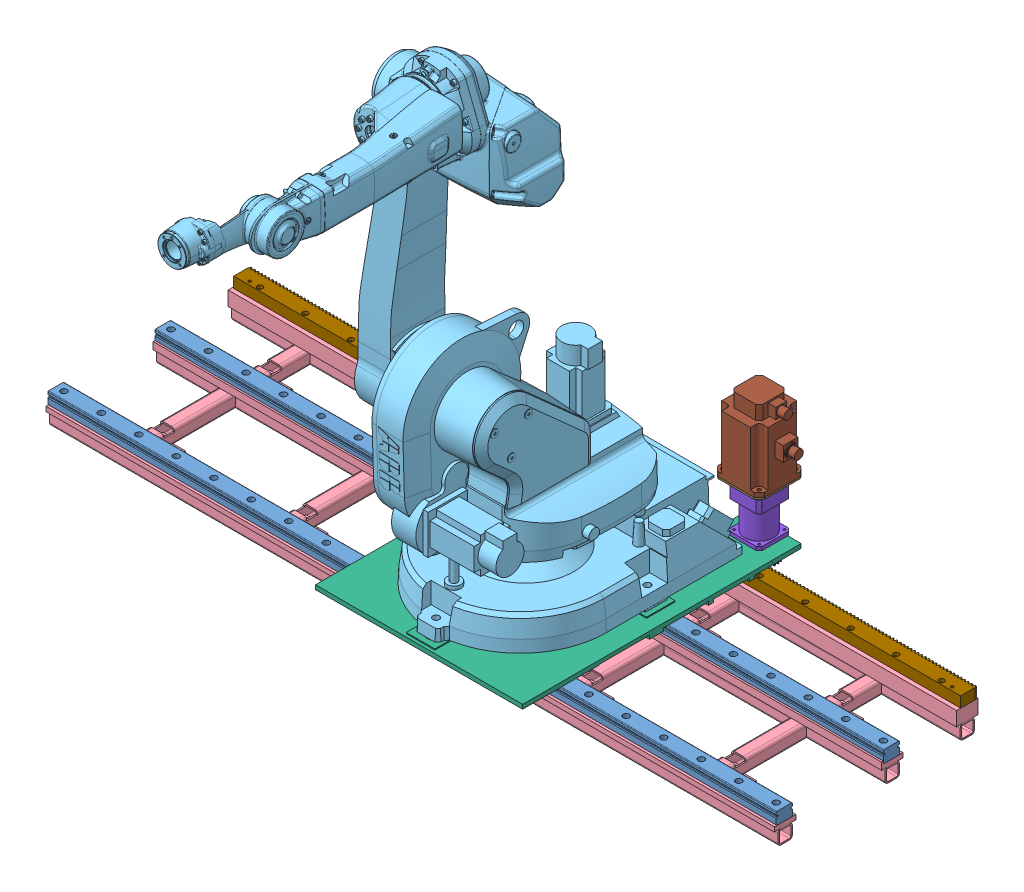
SolidWorks assembly 双导轨, configuration 默认. Lengths in mm.
Overall size (2040.11 1530 1501.91).
62 component instances, 12 part files, 57 mates.
Components (placement in the parent):
- 滑轨-1: 滑轨 [默认] at (-1407.5567 207.206 0) size (2040 34 45)
- 滑轨-2: 滑轨 [默认] at (632.4433 207.206 -300) x (-1 0 0) z (0 0 -1) size (2040 34 45)
- 带螺钉M4滑块-1: 带螺钉M4滑块 [默认] at (-58.6161 241.6075 -300) size (138.91 46.33 120)
  - 滑块-1: 滑块 [默认] at (-71.6389 25.5985 0) size (136 46 120)
  - cross recessed round head wood screws gb-2: cross recessed round head wood screws gb [GB_WOOD_SCREWS_TYPE136 M4X18-N] at (-74.5889 20.6207 -35.126) size (20.91 7.65 7.65)
  - cross recessed round head wood screws gb-4: cross recessed round head wood screws gb [GB_WOOD_SCREWS_TYPE136 M4X18-N] at (-74.5889 -15.566 -35.2553) size (20.91 7.65 7.65)
  - cross recessed round head wood screws gb-5: cross recessed round head wood screws gb [GB_WOOD_SCREWS_TYPE136 M4X18-N] at (-74.5889 20.0027 35.5979) size (20.91 7.65 7.65)
  - cross recessed round head wood screws gb-7: cross recessed round head wood screws gb [GB_WOOD_SCREWS_TYPE136 M4X18-N] at (-74.5889 -15.4341 35.4668) size (20.91 7.65 7.65)
  - cross recessed round head wood screws gb-8: cross recessed round head wood screws gb [GB_WOOD_SCREWS_TYPE136 M4X18-N] at (56.3111 20.1247 35.1143) x (-1 0 0) z (0 -0.924225 -0.381849) size (20.91 7.65 7.65)
  - cross recessed round head wood screws gb-9: cross recessed round head wood screws gb [GB_WOOD_SCREWS_TYPE136 M4X18-N] at (56.3111 -15.3216 35.4319) x (-1 0 0) z (0 -0.924225 -0.381849) size (20.91 7.65 7.65)
  - cross recessed round head wood screws gb-10: cross recessed round head wood screws gb [GB_WOOD_SCREWS_TYPE136 M4X18-N] at (56.3111 19.9496 -35.3218) x (-1 0 0) z (0 -0.924225 -0.381849) size (20.91 7.65 7.65)
  - cross recessed round head wood screws gb-11: cross recessed round head wood screws gb [GB_WOOD_SCREWS_TYPE136 M4X18-N] at (56.3111 -15.7298 -35.1914) x (-1 0 0) z (0 -0.924225 -0.381849) size (20.91 7.65 7.65)
- 带螺钉M4滑块-3: 带螺钉M4滑块 [默认] at (-58.6161 241.6075 0) size (138.91 46.33 120)
  - 滑块-1: 滑块 [默认] at (-71.6389 25.5985 0) size (136 46 120)
  - cross recessed round head wood screws gb-2: cross recessed round head wood screws gb [GB_WOOD_SCREWS_TYPE136 M4X18-N] at (-74.5889 20.6207 -35.126) size (20.91 7.65 7.65)
  - cross recessed round head wood screws gb-4: cross recessed round head wood screws gb [GB_WOOD_SCREWS_TYPE136 M4X18-N] at (-74.5889 -15.566 -35.2553) size (20.91 7.65 7.65)
  - cross recessed round head wood screws gb-5: cross recessed round head wood screws gb [GB_WOOD_SCREWS_TYPE136 M4X18-N] at (-74.5889 20.0027 35.5979) size (20.91 7.65 7.65)
  - cross recessed round head wood screws gb-7: cross recessed round head wood screws gb [GB_WOOD_SCREWS_TYPE136 M4X18-N] at (-74.5889 -15.4341 35.4668) size (20.91 7.65 7.65)
  - cross recessed round head wood screws gb-8: cross recessed round head wood screws gb [GB_WOOD_SCREWS_TYPE136 M4X18-N] at (56.3111 20.1247 35.1143) x (-1 0 0) z (0 -0.924225 -0.381849) size (20.91 7.65 7.65)
  - cross recessed round head wood screws gb-9: cross recessed round head wood screws gb [GB_WOOD_SCREWS_TYPE136 M4X18-N] at (56.3111 -15.3216 35.4319) x (-1 0 0) z (0 -0.924225 -0.381849) size (20.91 7.65 7.65)
  - cross recessed round head wood screws gb-10: cross recessed round head wood screws gb [GB_WOOD_SCREWS_TYPE136 M4X18-N] at (56.3111 19.9496 -35.3218) x (-1 0 0) z (0 -0.924225 -0.381849) size (20.91 7.65 7.65)
  - cross recessed round head wood screws gb-11: cross recessed round head wood screws gb [GB_WOOD_SCREWS_TYPE136 M4X18-N] at (56.3111 -15.7298 -35.1914) x (-1 0 0) z (0 -0.924225 -0.381849) size (20.91 7.65 7.65)
- 带螺钉M4滑块-4: 带螺钉M4滑块 [默认] at (-401.8938 241.6075 0) x (-1 0 0) z (0 0 -1) size (138.91 46.33 120)
  - 滑块-1: 滑块 [默认] at (-71.6389 25.5985 0) size (136 46 120)
  - cross recessed round head wood screws gb-2: cross recessed round head wood screws gb [GB_WOOD_SCREWS_TYPE136 M4X18-N] at (-74.5889 20.6207 -35.126) size (20.91 7.65 7.65)
  - cross recessed round head wood screws gb-4: cross recessed round head wood screws gb [GB_WOOD_SCREWS_TYPE136 M4X18-N] at (-74.5889 -15.566 -35.2553) size (20.91 7.65 7.65)
  - cross recessed round head wood screws gb-5: cross recessed round head wood screws gb [GB_WOOD_SCREWS_TYPE136 M4X18-N] at (-74.5889 20.0027 35.5979) size (20.91 7.65 7.65)
  - cross recessed round head wood screws gb-7: cross recessed round head wood screws gb [GB_WOOD_SCREWS_TYPE136 M4X18-N] at (-74.5889 -15.4341 35.4668) size (20.91 7.65 7.65)
  - cross recessed round head wood screws gb-8: cross recessed round head wood screws gb [GB_WOOD_SCREWS_TYPE136 M4X18-N] at (56.3111 20.1247 35.1143) x (-1 0 0) z (0 -0.924225 -0.381849) size (20.91 7.65 7.65)
  - cross recessed round head wood screws gb-9: cross recessed round head wood screws gb [GB_WOOD_SCREWS_TYPE136 M4X18-N] at (56.3111 -15.3216 35.4319) x (-1 0 0) z (0 -0.924225 -0.381849) size (20.91 7.65 7.65)
  - cross recessed round head wood screws gb-10: cross recessed round head wood screws gb [GB_WOOD_SCREWS_TYPE136 M4X18-N] at (56.3111 19.9496 -35.3218) x (-1 0 0) z (0 -0.924225 -0.381849) size (20.91 7.65 7.65)
  - cross recessed round head wood screws gb-11: cross recessed round head wood screws gb [GB_WOOD_SCREWS_TYPE136 M4X18-N] at (56.3111 -15.7298 -35.1914) x (-1 0 0) z (0 -0.924225 -0.381849) size (20.91 7.65 7.65)
- 带螺钉M4滑块-5: 带螺钉M4滑块 [默认] at (-401.8938 241.6075 -300) x (-1 0 0) z (0 0 -1) size (138.91 46.33 120)
  - 滑块-1: 滑块 [默认] at (-71.6389 25.5985 0) size (136 46 120)
  - cross recessed round head wood screws gb-2: cross recessed round head wood screws gb [GB_WOOD_SCREWS_TYPE136 M4X18-N] at (-74.5889 20.6207 -35.126) size (20.91 7.65 7.65)
  - cross recessed round head wood screws gb-4: cross recessed round head wood screws gb [GB_WOOD_SCREWS_TYPE136 M4X18-N] at (-74.5889 -15.566 -35.2553) size (20.91 7.65 7.65)
  - cross recessed round head wood screws gb-5: cross recessed round head wood screws gb [GB_WOOD_SCREWS_TYPE136 M4X18-N] at (-74.5889 20.0027 35.5979) size (20.91 7.65 7.65)
  - cross recessed round head wood screws gb-7: cross recessed round head wood screws gb [GB_WOOD_SCREWS_TYPE136 M4X18-N] at (-74.5889 -15.4341 35.4668) size (20.91 7.65 7.65)
  - cross recessed round head wood screws gb-8: cross recessed round head wood screws gb [GB_WOOD_SCREWS_TYPE136 M4X18-N] at (56.3111 20.1247 35.1143) x (-1 0 0) z (0 -0.924225 -0.381849) size (20.91 7.65 7.65)
  - cross recessed round head wood screws gb-9: cross recessed round head wood screws gb [GB_WOOD_SCREWS_TYPE136 M4X18-N] at (56.3111 -15.3216 35.4319) x (-1 0 0) z (0 -0.924225 -0.381849) size (20.91 7.65 7.65)
  - cross recessed round head wood screws gb-10: cross recessed round head wood screws gb [GB_WOOD_SCREWS_TYPE136 M4X18-N] at (56.3111 19.9496 -35.3218) x (-1 0 0) z (0 -0.924225 -0.381849) size (20.91 7.65 7.65)
  - cross recessed round head wood screws gb-11: cross recessed round head wood screws gb [GB_WOOD_SCREWS_TYPE136 M4X18-N] at (56.3111 -15.7298 -35.1914) x (-1 0 0) z (0 -0.924225 -0.381849) size (20.91 7.65 7.65)
- 焊架-1: 焊架 [默认<按加工>] at (-1407.5567 174.206 -302.5) x (1 0 0) z (0 1 0) size (2040 570 90)
- 机器人+工件台-1: 机器人+工件台 [默认] at (-235.255 279.206 -245) x (0 0 -1) z (0 1 0) size (1471.91 580 1415)
  - IRB1600ID_4_150__02_STEP_c-1: IRB1600ID_4_150__02_STEP_c [默认] at (-101.9143 0.2591 3) x (-1 0 0) z (0 0 1) size (1372.28 510.23 1392)
  - 工件台-2: 工件台 [默认] at (-50 0 -20) x (1 0 0) z (0 -1 0) size (780 23 580)
- slotted set screws with cone point gb-18: slotted set screws with cone point gb [GB_FASTENER_SCREWS_NCOB M4X16-S] at (-90.255 263.206 -376) x (0 0 1) z (0.748487 -0.66315 0) size (15.99 4 4)
- slotted set screws with cone point gb-16: slotted set screws with cone point gb [GB_FASTENER_SCREWS_NCOB M4X16-S] at (-30.255 263.206 -376) x (0 0 1) z (0.08595 -0.996299 0) size (15.99 4 4)
- slotted set screws with cone point gb-15: slotted set screws with cone point gb [GB_FASTENER_SCREWS_NCOB M4X16-S] at (-50.255 263.206 -376) x (0 0 1) z (-0.998235 -0.059386 0) size (15.99 4 4)
- slotted set screws with cone point gb-13: slotted set screws with cone point gb [GB_FASTENER_SCREWS_NCOB M4X16-S] at (-70.255 263.206 -376) x (0 0 1) z (-0.354194 -0.935172 0) size (15.99 4 4)
- slotted set screws with cone point gb-11: slotted set screws with cone point gb [GB_FASTENER_SCREWS_NCOB M4X16-S] at (-110.255 263.206 -376) x (0 0 1) z (-0.974836 -0.222922 0) size (15.99 4 4)
- slotted set screws with cone point gb-10: slotted set screws with cone point gb [GB_FASTENER_SCREWS_NCOB M4X16-S] at (-435.255 263.206 -376) x (0 0 1) z (-0.993007 0.118057 0) size (15.99 4 4)
- slotted set screws with cone point gb-9: slotted set screws with cone point gb [GB_FASTENER_SCREWS_NCOB M4X16-S] at (-415.255 263.206 -376) x (0 0 1) z (-0.998721 -0.050563 0) size (15.99 4 4)
- slotted set screws with cone point gb-7: slotted set screws with cone point gb [GB_FASTENER_SCREWS_NCOB M4X16-S] at (-395.255 263.206 -376) x (0 0 1) z (-1 0 0) size (15.99 4 4)
- slotted set screws with cone point gb-4: slotted set screws with cone point gb [GB_FASTENER_SCREWS_NCOB M4X16-S] at (-375.255 263.206 -376) x (0 0 1) z (-0.982111 0.188301 0) size (15.99 4 4)
- slotted set screws with cone point gb-2: slotted set screws with cone point gb [GB_FASTENER_SCREWS_NCOB M4X16-S] at (-355.255 263.206 -376) x (0 0 1) z (-0.85186 0.52377 0) size (15.99 4 4)
- PLE8090级数2减速比15-1: PLE8090级数2减速比15 [默认] at (-22.7544 284.206 -585) x (0 -1 0) z (1 0 0) size (162.5 90 90)
- 齿条-2: 齿条 [默认] at (-385.4567 234.206 -494) x (1 0 0) z (0 1 0) size (1018.01 46 30)
- 齿轮-CSGH030322-2: 齿轮-CSGH030322 [默认] at (-22.7544 263.206 -585) x (0.526718 0 0.85004) z (0 -1 0) size (101.69 101.69 30)
- 齿条-3: 齿条 [默认] at (-1403.3567 234.206 -494) x (1 0 0) z (0 1 0) size (1018.01 46 30)
- HC-SFS1524B-1: HC-SFS1524B [默认] at (-22.7544 579.4989 -520) x (0 -1 0) z (0 0 -1) size (258 176 130)
- 法兰盘-1: 法兰盘 [默认] at (-22.7544 430.206 -585) x (0 -1 0) z (0 0 1) size (23.5 130 130)
Mates (geometry in assembly coordinates):
- 距离1: distance = 300 mm aligned: plane of 滑轨-1 through (632.4433 209.206 22.5) normal (0 0 1); plane of 滑轨-2 through (-1407.5567 209.206 -277.5) normal (0 0 1)
- 重合2: coincident aligned: plane of 滑轨-1 through (632.4433 241.206 -20.5) normal (0 1 0); plane of 滑轨-2 through (-1407.5567 241.206 -279.5) normal (0 1 0)
- 重合3: coincident aligned: plane of 滑轨-1 through (-1407.5567 239.206 -20.5) normal (-1 0 0); plane of 滑轨-2 through (-1407.5567 239.206 -279.5) normal (-1 0 0)
- 重合4: coincident anti-aligned: plane of 滑轨-2 through (-1407.5567 241.206 -279.5) normal (0 1 0); plane of 带螺钉M4滑块-1/滑块-1 through (-5.255 241.206 -321) normal (0 -1 0)
- 距离2: distance = 37.5 mm aligned: plane of 带螺钉M4滑块-1/滑块-1 through (-5.255 265.206 -360) normal (0 0 -1); plane of 滑轨-2 through (-1407.5567 209.206 -322.5) normal (0 0 -1)
- 重合10: coincident aligned: plane of 带螺钉M4滑块-1/滑块-1 through (-5.255 233.206 -321) normal (1 0 0); plane of 带螺钉M4滑块-3/滑块-1 through (-5.255 233.206 -21) normal (1 0 0)
- 距离6: distance = 60 mm anti-aligned: plane of 带螺钉M4滑块-3/滑块-1 through (-5.255 267.206 58) normal (0 1 0); plane of 滑轨-1 through (632.4433 207.206 20.5) normal (0 -1 0)
- 距离7: distance = 37.5 mm aligned: plane of 带螺钉M4滑块-3/滑块-1 through (-5.255 265.206 60) normal (0 0 1); plane of 滑轨-1 through (632.4433 209.206 22.5) normal (0 0 1)
- 距离8: distance = 200 mm anti-aligned: plane of 带螺钉M4滑块-4/滑块-1 through (-330.255 233.206 21) normal (1 0 0); plane of 带螺钉M4滑块-3/滑块-1 through (-130.255 233.206 -21) normal (-1 0 0)
- 距离9: distance = 60 mm anti-aligned: plane of 带螺钉M4滑块-4/滑块-1 through (-455.255 267.206 -58) normal (0 1 0); plane of 滑轨-1 through (632.4433 207.206 20.5) normal (0 -1 0)
- 距离10: distance = 37.5 mm aligned: plane of 带螺钉M4滑块-4/滑块-1 through (-455.255 265.206 60) normal (0 0 1); plane of 滑轨-1 through (632.4433 209.206 22.5) normal (0 0 1)
- 重合16: coincident aligned: plane of 带螺钉M4滑块-4/滑块-1 through (-330.255 233.206 21) normal (1 0 0); plane of 带螺钉M4滑块-5/滑块-1 through (-330.255 233.206 -279) normal (1 0 0)
- 重合17: coincident aligned: plane of 带螺钉M4滑块-4/滑块-1 through (-455.255 267.206 -58) normal (0 1 0); plane of 带螺钉M4滑块-5/滑块-1 through (-455.255 267.206 -358) normal (0 1 0)
- 重合18: coincident aligned: plane of 带螺钉M4滑块-1/滑块-1 through (-5.255 265.206 -240) normal (0 0 1); plane of 带螺钉M4滑块-5/滑块-1 through (-455.255 265.206 -240) normal (0 0 1)
- 重合19: coincident anti-aligned: plane of 滑轨-2 through (-1407.5567 207.206 -320.5) normal (0 -1 0); plane of 焊架-1 through (632.4443 207.206 -277.5) normal (0 1 0)
- 重合20: coincident anti-aligned: plane of 滑轨-2 through (-1407.5567 209.206 -277.5) normal (0 0 1); plane of 焊架-1 through (632.4443 214.206 -277.5) normal (0 0 -1)
- 重合21: coincident aligned: plane of 滑轨-2 through (-1407.5567 239.206 -279.5) normal (-1 0 0); plane of 焊架-1 through (-1407.5567 174.206 -302.5) normal (-1 0 0)
- 距离14: distance = 70 mm aligned: plane of 机器人+工件台-1/工件台-2 through (-525.255 279.206 -545) normal (-1 0 0); plane of 带螺钉M4滑块-5/滑块-1 through (-455.255 233.206 -279) normal (-1 0 0)
- 重合39: coincident anti-aligned: plane of 带螺钉M4滑块-5/滑块-1 through (-455.255 265.206 -240) normal (0 0 1); plane of 机器人+工件台-1/工件台-2 through (54.7466 266.1454 -240) normal (0 0 -1)
- 同心2: concentric aligned: cylinder of 机器人+工件台-1/工件台-2 through (-355.255 263.206 155.001) axis (0 0 -1) radius 2; cylinder of slotted set screws with cone point gb-2 through (-355.255 263.206 -384.5703) axis (0 0 -1) radius 2
- 同心31: concentric aligned: cylinder of 机器人+工件台-1/工件台-2 through (-375.255 263.206 155.001) axis (0 0 -1) radius 2; cylinder of slotted set screws with cone point gb-4 through (-375.255 263.206 -384.5703) axis (0 0 -1) radius 2
- 同心7: concentric aligned: cylinder of 机器人+工件台-1/工件台-2 through (-415.255 263.206 155.001) axis (0 0 -1) radius 2; cylinder of slotted set screws with cone point gb-9 through (-415.255 263.206 -384.5703) axis (0 0 -1) radius 2
- 同心8: concentric aligned: cylinder of 机器人+工件台-1/工件台-2 through (-435.255 263.206 155.001) axis (0 0 -1) radius 2; cylinder of slotted set screws with cone point gb-10 through (-435.255 263.206 -384.5703) axis (0 0 -1) radius 2
- 同心9: concentric aligned: cylinder of 机器人+工件台-1/工件台-2 through (-110.255 263.206 155.001) axis (0 0 -1) radius 2; cylinder of slotted set screws with cone point gb-11 through (-110.255 263.206 -384.5703) axis (0 0 -1) radius 2
- 同心10: concentric aligned: cylinder of 机器人+工件台-1/工件台-2 through (-70.255 263.206 155.001) axis (0 0 -1) radius 2; cylinder of slotted set screws with cone point gb-13 through (-70.255 263.206 -384.5703) axis (0 0 -1) radius 2
- 同心12: concentric aligned: cylinder of 机器人+工件台-1/工件台-2 through (-50.255 263.206 155.001) axis (0 0 -1) radius 2; cylinder of slotted set screws with cone point gb-15 through (-50.255 263.206 -384.5703) axis (0 0 -1) radius 2
- 同心13: concentric aligned: cylinder of 机器人+工件台-1/工件台-2 through (-30.255 263.206 155.001) axis (0 0 -1) radius 2; cylinder of slotted set screws with cone point gb-16 through (-30.255 263.206 -384.5703) axis (0 0 -1) radius 2
- 同心14: concentric aligned: cylinder of 机器人+工件台-1/工件台-2 through (-90.255 263.206 155.001) axis (0 0 -1) radius 2; cylinder of slotted set screws with cone point gb-18 through (-90.255 263.206 -384.5703) axis (0 0 -1) radius 2
- 重合41: coincident anti-aligned: plane of 带螺钉M4滑块-5/滑块-1 through (-455.255 265.206 -360) normal (0 0 -1); circle of slotted set screws with cone point gb-10
- 重合42: coincident anti-aligned: plane of 带螺钉M4滑块-5/滑块-1 through (-455.255 265.206 -360) normal (0 0 -1); plane of slotted set screws with cone point gb-9 through (-415.255 263.206 -360) normal (0 0 1)
- 重合43: coincident anti-aligned: plane of 带螺钉M4滑块-5/滑块-1 through (-455.255 265.206 -360) normal (0 0 -1); plane of slotted set screws with cone point gb-7 through (-395.255 263.206 -360) normal (0 0 1)
- 重合44: coincident anti-aligned: plane of 带螺钉M4滑块-5/滑块-1 through (-455.255 265.206 -360) normal (0 0 -1); circle of slotted set screws with cone point gb-4
- 重合45: coincident anti-aligned: plane of 带螺钉M4滑块-5/滑块-1 through (-455.255 265.206 -360) normal (0 0 -1); circle of slotted set screws with cone point gb-2
- 重合46: coincident anti-aligned: plane of 带螺钉M4滑块-1/滑块-1 through (-5.255 265.206 -360) normal (0 0 -1); circle of slotted set screws with cone point gb-11
- 重合47: coincident anti-aligned: plane of 带螺钉M4滑块-1/滑块-1 through (-5.255 265.206 -360) normal (0 0 -1); circle of slotted set screws with cone point gb-18
- 重合48: coincident anti-aligned: plane of 带螺钉M4滑块-1/滑块-1 through (-5.255 265.206 -360) normal (0 0 -1); plane of slotted set screws with cone point gb-13 through (-70.255 263.206 -360) normal (0 0 1)
- 重合49: coincident anti-aligned: plane of 带螺钉M4滑块-1/滑块-1 through (-5.255 265.206 -360) normal (0 0 -1); plane of slotted set screws with cone point gb-15 through (-50.255 263.206 -360) normal (0 0 1)
- 重合50: coincident anti-aligned: plane of 带螺钉M4滑块-1/滑块-1 through (-5.255 265.206 -360) normal (0 0 -1); circle of slotted set screws with cone point gb-16
- 同心15: concentric anti-aligned: circle of 机器人+工件台-1/工件台-2; circle of slotted set screws with cone point gb-7
- 同心32: concentric aligned: cylinder of 机器人+工件台-1/工件台-2 through (-22.7544 259.205 -585) axis (0 1 0) radius 20; cylinder of PLE8090级数2减速比15-1 through (-22.7544 337.7324 -585) axis (0 1 0) radius 10
- 重合59: coincident anti-aligned: plane of 机器人+工件台-1/工件台-2 through (-235.255 279.206 -195) normal (0 1 0); plane of PLE8090级数2减速比15-1 through (-22.7544 279.206 -602.5) normal (0 -1 0)
- 重合74: coincident anti-aligned: plane of 焊架-1 through (-1407.5567 234.206 -542.5) normal (0 1 0); plane of 齿条-2 through (-385.4567 234.206 -494) normal (0 -1 0)
- 重合75: coincident aligned: plane of 齿条-2 through (632.4433 264.206 -494) normal (1 0 0); plane of 焊架-1 through (632.4433 174.206 -302.5) normal (1 0 0)
- 距离16: distance = 1 mm aligned: plane of 齿轮-CSGH030322-2 through (-22.7544 263.206 -585) normal (0 1 0); plane of 齿条-2 through (-385.4567 264.206 -494) normal (0 1 0)
- 同心34: concentric aligned: cylinder of 机器人+工件台-1/工件台-2 through (-22.7544 259.205 -585) axis (0 1 0) radius 20; cylinder of 齿轮-CSGH030322-2 through (-22.7544 234.205 -585) axis (0 1 0) radius 15
- 相切3: tangent anti-aligned: plane of 齿条-2 through (-385.4567 264.206 -534) normal (0 0 -1); cylinder of 齿轮-CSGH030322-2 through (-22.7544 235.206 -585) axis (0 1 0) radius 51
- 重合76: coincident anti-aligned: plane of 齿条-2 through (-385.4567 264.206 -494) normal (-1 0 0); plane of 齿条-3 through (-385.4567 264.206 -494) normal (1 0 0)
- 重合77: coincident anti-aligned: plane of 焊架-1 through (-1407.5567 234.206 -542.5) normal (0 1 0); plane of 齿条-3 through (-1403.3567 234.206 -494) normal (0 -1 0)
- 重合78: coincident aligned: plane of 齿条-2 through (-385.4567 264.206 -494) normal (0 0 1); plane of 齿条-3 through (-1403.3567 264.206 -494) normal (0 0 1)
- 平行1: parallel aligned: plane of 机器人+工件台-1/工件台-2 through (-235.255 267.206 -625) normal (0 0 -1); plane of PLE8090级数2减速比15-1 through (13.8379 294.206 -630) normal (0 0 -1)
- 重合93: coincident anti-aligned: plane of PLE8090级数2减速比15-1 through (-22.7544 406.706 -585) normal (0 1 0); plane of 法兰盘-1 through (-22.7544 406.706 -585) normal (0 -1 0)
- 同心43: concentric anti-aligned: cylinder of PLE8090级数2减速比15-1 through (-22.7544 376.706 -585) axis (0 1 0) radius 7; cylinder of 法兰盘-1 through (-22.7544 430.206 -585) axis (0 -1 0) radius 12
- 同心44: concentric anti-aligned: cylinder of HC-SFS1524B-1 through (-22.7544 375.206 -585) axis (0 1 0) radius 12; cylinder of 法兰盘-1 through (-22.7544 430.206 -585) axis (0 -1 0) radius 12
- 重合94: coincident anti-aligned: plane of HC-SFS1524B-1 through (-87.7544 430.206 -650) normal (0 -1 0); plane of 法兰盘-1 through (-22.7544 430.206 -585) normal (0 1 0)
- 平行2: parallel aligned: plane of PLE8090级数2减速比15-1 through (13.8379 294.206 -630) normal (0 0 -1); plane of 法兰盘-1 through (-73.5604 425.206 -650) normal (0 0 -1)
- 同心45: concentric anti-aligned: cylinder of HC-SFS1524B-1 through (28.5108 633.207 -533.7348) axis (0 -1 0) radius 4.5; cylinder of 法兰盘-1 through (28.5108 425.206 -533.7348) axis (0 1 0) radius 4.5
- 重合96: coincident anti-aligned: plane of 带螺钉M4滑块-5/滑块-1 through (-455.255 267.206 -358) normal (0 1 0); plane of 机器人+工件台-1/工件台-2 through (54.7466 267.206 -360) normal (0 -1 0)
